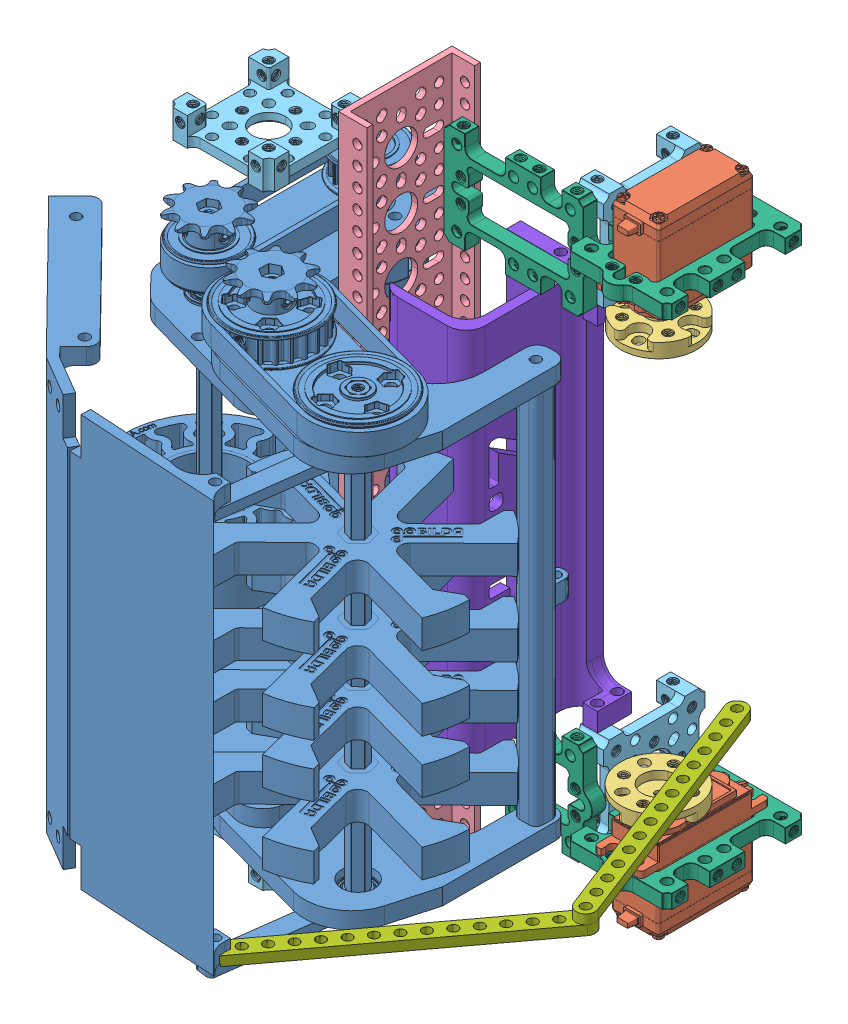
SolidWorks assembly Intake Sub-Assembly League Champs, configuration Default. Lengths in mm.
Overall size (212.49 288 206.87).
17 component instances, 8 part files, 47 mates.
Components (placement in the parent):
- Intake Sub-Assembly League Meet 5-1: Intake Sub-Assembly League Meet 5 [Default] at (116.6856 190.4437 282.0958) size (196.76 202.81 172.35)
- servo.step-1: servo.step [Default] at (176.6285 91.3596 206.3723) x (0 0 -1) z (0 1 0) size (54.3 20 43.9)
- servo.step-4: servo.step [Default] at (176.7285 278.9596 206.3723) x (0 0 -1) z (0 -1 0) size (54.3 20 43.9)
- 1908-0025-0032.step-1: 1908-0025-0032.step [Default] at (176.7285 276.6596 216.2223) x (-0.858745 0 -0.512404) z (-0.512404 0 0.858745) size (31.98 8 31.98)
- 1908-0025-0032.step-2: 1908-0025-0032.step [Default] at (176.6285 93.6596 216.2223) x (0.932599 0 -0.360915) z (0.360915 0 0.932599) size (31.98 8 31.98)
- 11 Hole Low-Side U Channel 288mm.step-1: 11 Hole Low-Side U Channel 288mm.step [Default] at (110.1785 37.1596 258.6223) size (12 288 48)
- quad block.step-3: quad block.step [Default] at (64.6785 309.1596 269.1223) size (43.01 12.01 43.01)
- quad block.step-4: quad block.step [Default] at (64.6785 65.1596 269.1223) x (1 0 0) z (0 0 -1) size (43.01 12.01 43.01)
- servo mount-1: servo mount [Default] at (156.1362 300.8003 219.8855) x (1 0 0) z (0 -1 0) size (62.75 6.01 43)
- servo mount-3: servo mount [Default] at (156.1362 100.8003 219.8855) x (1 0 0) z (0 -1 0) size (62.75 6.01 43)
- quad block.step-5: quad block.step [Default] at (155.1785 85.1596 196.6223) x (0 1 0) z (0 0 1) size (43.01 12.01 43.01)
- quad block.step-6: quad block.step [Default] at (155.1785 285.1596 196.6223) x (0 1 0) z (0 0 1) size (43.01 12.01 43.01)
- servo mount-4: servo mount [Default] at (192.3192 291.9228 237.58) x (0 0 1) z (-1 0 0) size (62.75 6.01 43)
- servo mount-5: servo mount [Default] at (192.3192 75.9228 237.58) x (0 0 1) z (-1 0 0) size (62.75 6.01 43)
- 15 hole flat beam.step-1: 15 hole flat beam.step [Default] at (189.8639 101.6596 228.2565) x (0.360915 0 0.932599) z (-0.932599 0 0.360915) size (120 4 8)
- 15 hole flat beam.step-2: 15 hole flat beam.step [Default] at (176.6404 97.6596 325.4056) x (0.597049 0 -0.802205) z (0.802205 0 0.597049) size (120 4 8)
- Wire Cover-1: Wire Cover [Default] at (147.1785 106.6596 212.6223) x (-1 0 0) z (0 0 -1) size (52 157 54)
Mates (geometry in assembly coordinates):
- Coincident51: coincident anti-aligned: plane of Intake Sub-Assembly League Meet 5-1 through (86.1785 257.6596 359.7719) normal (1 0 0); plane of 11 Hole Low-Side U Channel 288mm.step-1 through (86.1785 325.1596 213.1223) normal (-1 0 0)
- Concentric31: concentric anti-aligned: cylinder of Intake Sub-Assembly League Meet 5-1 through (79.3785 261.1596 221.1223) axis (1 0 0) radius 3.175; cylinder of 11 Hole Low-Side U Channel 288mm.step-1 through (96.1785 261.1596 221.1223) axis (-1 0 0) radius 2
- Parallel1: parallel aligned: plane of Intake Sub-Assembly League Meet 5-1 through (96.8429 106.6596 205.3723) normal (0 0 -1); plane of 11 Hole Low-Side U Channel 288mm.step-1 through (88.6785 325.1596 213.1223) normal (0 0 -1)
- Concentric42: concentric anti-aligned: circle of servo.step-4; cylinder of 1908-0025-0032.step-1 through (176.7285 268.6596 216.2223) axis (0 1 0) radius 15.99
- Coincident62: coincident anti-aligned: plane of servo.step-4 through (176.7285 273.2596 216.2223) normal (0 -1 0); plane of 1908-0025-0032.step-1 through (176.7285 273.2596 216.2223) normal (0 1 0)
- Coincident63: coincident anti-aligned: plane of servo.step-1 through (176.6285 97.0596 216.2223) normal (0 1 0); plane of 1908-0025-0032.step-2 through (176.6285 97.0596 216.2223) normal (0 -1 0)
- Tangent1: tangent: plane of 11 Hole Low-Side U Channel 288mm.step-1 through (96.1785 59.1596 253.1223) normal (0 1 0); circle of quad block.step-4
- Coincident67: coincident anti-aligned: plane of 11 Hole Low-Side U Channel 288mm.step-1 through (86.1785 325.1596 213.1223) normal (-1 0 0); plane of quad block.step-4 through (86.1785 61.1596 269.1223) normal (1 0 0)
- Parallel2: parallel aligned: plane of 11 Hole Low-Side U Channel 288mm.step-1 through (110.1785 37.1596 258.6223) normal (0 -1 0); plane of quad block.step-4 through (64.6785 61.1596 269.1223) normal (0 -1 0)
- Tangent2: tangent: cylinder of 11 Hole Low-Side U Channel 288mm.step-1 through (96.1785 53.1596 253.1223) axis (-1 0 0) radius 2; circle of quad block.step-4
- Coincident69: coincident aligned: cylinder of 11 Hole Low-Side U Channel 288mm.step-1 through (96.1785 317.1596 253.1223) axis (-1 0 0) radius 2; circle of quad block.step-3
- Coincident70: coincident anti-aligned: plane of 11 Hole Low-Side U Channel 288mm.step-1 through (86.1785 325.1596 213.1223) normal (-1 0 0); plane of quad block.step-3 through (86.1785 313.1596 269.1223) normal (1 0 0)
- Parallel3: parallel aligned: plane of 11 Hole Low-Side U Channel 288mm.step-1 through (110.1785 325.1596 258.6223) normal (0 1 0); plane of quad block.step-3 through (64.6785 313.1596 269.1223) normal (0 1 0)
- Concentric44: concentric anti-aligned: cylinder of 11 Hole Low-Side U Channel 288mm.step-1 through (96.1785 301.1596 221.1223) axis (-1 0 0) radius 2; circle of servo mount-1
- Parallel4: parallel aligned: plane of 11 Hole Low-Side U Channel 288mm.step-1 through (88.6785 325.1596 213.1223) normal (0 0 -1); plane of servo mount-1 through (125.1785 285.1596 218.1223) normal (0 0 -1)
- Parallel5: parallel aligned: plane of 11 Hole Low-Side U Channel 288mm.step-1 through (88.6785 325.1596 213.1223) normal (0 0 -1); plane of servo mount-3 through (125.1785 85.1596 218.1223) normal (0 0 -1)
- Concentric47: concentric anti-aligned: circle of 11 Hole Low-Side U Channel 288mm.step-1; circle of servo mount-3
- Coincident74: coincident aligned: plane of servo mount-1 through (152.6785 285.1596 218.1223) normal (1 0 0); plane of servo mount-3 through (152.6785 85.1596 218.1223) normal (1 0 0)
- Distance2: distance = 5 mm anti-aligned: plane of 11 Hole Low-Side U Channel 288mm.step-1 through (88.6785 325.1596 258.6223) normal (1 0 0); plane of servo mount-3 through (93.6785 85.1596 224.1223) normal (-1 0 0)
- Concentric48: concentric aligned: cylinder of servo.step-1 through (176.6285 93.0596 216.2223) axis (0 -1 0) radius 5.45; cylinder of 1908-0025-0032.step-2 through (176.6285 101.6596 216.2223) axis (0 -1 0) radius 15.99
- Concentric49: concentric aligned: cylinder of servo mount-3 through (147.1785 101.1596 204.5208) axis (0 0 1) radius 2.025; circle of quad block.step-5
- Coincident75: coincident anti-aligned: plane of servo mount-3 through (125.1785 85.1596 218.1223) normal (0 0 -1); plane of quad block.step-5 through (164.3709 85.1596 218.1223) normal (0 0 1)
- Parallel6: parallel aligned: plane of servo mount-3 through (152.6785 85.1596 218.1223) normal (1 0 0); plane of quad block.step-5 through (155.1785 85.1596 196.6223) normal (1 0 0)
- Concentric50: concentric aligned: cylinder of servo mount-1 through (147.1785 301.1596 204.5208) axis (0 0 1) radius 2.025; circle of quad block.step-6
- Coincident77: coincident anti-aligned: plane of servo mount-1 through (125.1785 285.1596 218.1223) normal (0 0 -1); plane of quad block.step-6 through (164.3709 285.1596 218.1223) normal (0 0 1)
- Parallel7: parallel aligned: plane of servo mount-1 through (152.6785 285.1596 218.1223) normal (1 0 0); plane of quad block.step-6 through (155.1785 285.1596 196.6223) normal (1 0 0)
- Coincident78: coincident anti-aligned: plane of quad block.step-6 through (155.1785 285.1596 196.6223) normal (1 0 0); plane of servo mount-4 through (155.1785 296.1596 206.6223) normal (-1 0 0)
- Concentric53: concentric anti-aligned: cylinder of quad block.step-5 through (151.1785 77.1596 180.6223) axis (-1 0 0) radius 2; circle of servo mount-5
- Concentric54: concentric anti-aligned: cylinder of quad block.step-5 through (151.1785 77.1596 212.6223) axis (-1 0 0) radius 2; circle of servo mount-5
- Coincident79: coincident anti-aligned: plane of quad block.step-5 through (155.1785 85.1596 196.6223) normal (1 0 0); plane of servo mount-5 through (155.1785 80.1596 206.6223) normal (-1 0 0)
- Concentric55: concentric aligned: cylinder of quad block.step-6 through (151.1785 293.1596 180.6223) axis (-1 0 0) radius 2; circle of servo mount-4
- Parallel8: parallel aligned: plane of quad block.step-6 through (151.1785 266.1596 196.6223) normal (0 -1 0); plane of servo mount-4 through (176.6785 290.1596 206.6223) normal (0 -1 0)
- Concentric56: concentric aligned: cylinder of servo.step-4 through (181.6785 290.1606 182.3723) axis (0 -1 0) radius 2.25; circle of servo mount-4
- Coincident81: coincident anti-aligned: plane of servo.step-4 through (185.2285 290.1596 180.7223) normal (0 1 0); plane of servo mount-4 through (176.6785 290.1596 206.6223) normal (0 -1 0)
- Parallel9: parallel aligned: plane of servo.step-4 through (186.7285 290.1596 186.9223) normal (1 0 0); plane of servo mount-4 through (190.1785 296.1596 206.6223) normal (1 0 0)
- Concentric57: concentric aligned: cylinder of servo.step-1 through (171.6785 80.1586 182.3723) axis (0 1 0) radius 2.25; circle of servo mount-5
- Coincident83: coincident anti-aligned: plane of servo.step-1 through (168.1285 80.1596 180.7223) normal (0 -1 0); plane of servo mount-5 through (176.6785 80.1596 206.6223) normal (0 1 0)
- Parallel10: parallel aligned: plane of servo.step-1 through (186.6285 80.1596 186.9223) normal (1 0 0); plane of servo mount-5 through (190.1785 80.1596 206.6223) normal (1 0 0)
- Coincident85: coincident anti-aligned: plane of 1908-0025-0032.step-2 through (176.6285 101.6596 216.2223) normal (0 1 0); plane of 15 hole flat beam.step-1 through (169.6527 101.6596 176.031) normal (0 -1 0)
- Concentric60: concentric anti-aligned: cylinder of Intake Sub-Assembly League Meet 5-1 through (143.2057 105.5872 370.329) axis (0 -1 0) radius 2.05; cylinder of 15 hole flat beam.step-2 through (143.2057 101.6596 370.329) axis (0 1 0) radius 2
- Concentric61: concentric aligned: cylinder of 15 hole flat beam.step-1 through (210.0752 105.6596 280.4821) axis (0 1 0) radius 2; cylinder of 15 hole flat beam.step-2 through (210.0752 101.6596 280.4821) axis (0 1 0) radius 2
- Coincident88: coincident anti-aligned: plane of 15 hole flat beam.step-1 through (169.6527 101.6596 176.031) normal (0 -1 0); plane of 15 hole flat beam.step-2 through (143.2057 101.6596 370.329) normal (0 1 0)
- Concentric62: concentric anti-aligned: cylinder of 1908-0025-0032.step-2 through (181.202 101.6596 205.8742) axis (0 -1 0) radius 2; cylinder of 15 hole flat beam.step-1 through (181.202 105.6596 205.8742) axis (0 1 0) radius 2
- Concentric63: concentric anti-aligned: cylinder of 1908-0025-0032.step-2 through (186.9766 101.6596 220.7957) axis (0 -1 0) radius 2; cylinder of 15 hole flat beam.step-1 through (186.9766 105.6596 220.7957) axis (0 1 0) radius 2
- Coincident91: coincident anti-aligned: plane of servo mount-1 through (125.1785 263.6596 224.1223) normal (0 -1 0); plane of Wire Cover-1 through (147.1785 263.6596 212.6223) normal (0 1 0)
- Parallel12: parallel anti-aligned: plane of servo mount-5 through (176.6785 80.1596 175.1223) normal (0 0 -1); plane of Wire Cover-1 through (144.1785 263.6596 215.6223) normal (0 0 1)
- Concentric65: concentric anti-aligned: circle of quad block.step-5; cylinder of Wire Cover-1 through (147.1785 263.6596 212.6223) axis (0 -1 0) radius 2.1
